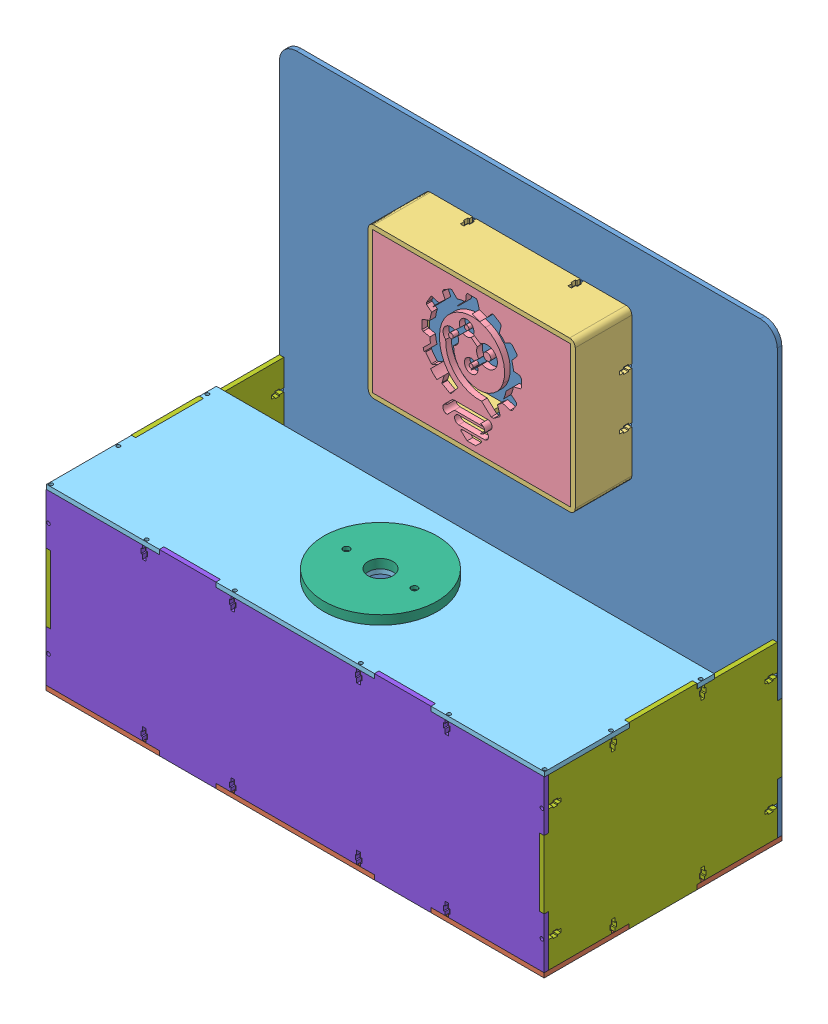
SolidWorks assembly Assemblage1, configuration Défaut. Lengths in mm.
Overall size (440.38 394 210).
10 component instances, 9 part files, 23 mates.
Components (placement in the parent):
- Pièce1-1: Pièce1 [Défaut] at origin size (440 394 4)
- Pièce2-1: Pièce2 [Défaut] at (0 -195 105) x (-1 0 0) z (0 -1 0) size (440 210 4)
- Pièce4-1: Pièce4 [Défaut] at (0 79.5409 54) x (1 0 0) z (0 0 -1) size (243.14 184.79 50)
- Part10 - Copie-1: Part10 - Copie [Default] at (-51.8221 -2.5899 50.5) size (175 125 11.52)
- Pièce7-1: Pièce7 [Défaut] at (0.3751 -41 135) x (1 0 0) z (0 -1 0) size (440 150 4)
- Pièce8-1: Pièce8 [Défaut] at (0.3751 -33 135) x (1 0 0) z (0 -1 0) size (100 100 8)
- Pièce9-1: Pièce9 [Défaut] at (-220 -120 105) x (0 0 -1) z (1 0 0) size (210 158 4)
- Pièce9-2: Pièce9 [Défaut] at (216 -120 105) x (0 0 -1) z (1 0 0) size (210 158 4)
- Pièce6-2: Pièce6 [Défaut] at (0 -120 206) size (440 158 4)
- ArduinoUno complet-1: ArduinoUno complet [Défaut] at (-169.33 -195 106.04) x (0 0 -1) z (1 0 0) size (76.34 15.58 53.34)
Mates (geometry in assembly coordinates):
- Coïncidente1: coincident anti-aligned: plane of Pièce1-1 through (220 -195 4) normal (0 -1 0); plane of Pièce2-1 through (0 -195 105) normal (0 1 0)
- Coïncidente2: coincident aligned: plane of Pièce1-1 through (0 0 0) normal (0 0 -1); plane of Pièce2-1 through (-220 -199 0) normal (0 0 -1)
- Largeur1: width aligned: plane of Pièce2-1 through (220 -199 210) normal (1 0 0); plane of Pièce2-1 through (-220 -199 210) normal (-1 0 0); plane of Pièce1-1 through (220 -195 4) normal (1 0 0); plane of Pièce1-1 through (-220 -195 4) normal (-1 0 0)
- Coïncidente5: coincident anti-aligned: plane of Pièce1-1 through (0 0 4) normal (0 0 1); plane of Pièce4-1 through (0 79.5409 4) normal (0 0 -1)
- Parallèle1: parallel aligned: plane of Pièce2-1 through (0 -195 105) normal (0 1 0); plane of Pièce4-1 through (91.5 146.0409 4) normal (0 1 0)
- Largeur2: width aligned: plane of Pièce1-1 through (-220 -195 4) normal (-1 0 0); plane of Pièce1-1 through (220 -195 4) normal (1 0 0); plane of Pièce4-1 through (-91.5 146.0409 4) normal (-1 0 0); plane of Pièce4-1 through (91.5 146.0409 4) normal (1 0 0)
- Coïncidente7: coincident anti-aligned: plane of Pièce4-1 through (-85.9962 142.0409 4) normal (0 -1 0); plane of Part10 - Copie-1 through (-87.5 142.0409 49) normal (0 1 0)
- Coïncidente8: coincident aligned: plane of Pièce4-1 through (0 79.5409 54) normal (0 0 1); plane of Part10 - Copie-1 through (-51.8221 -2.5899 54) normal (0 0 1)
- Coïncidente9: coincident: plane of Pièce4-1 through (-87.5 142.0409 4) normal (1 0 0); line of Part10 - Copie-1 through (-87.5 17.0409 54) axis (0 1 0)
- Coïncidente23: coincident anti-aligned: plane of Pièce7-1 through (0.3751 -41 135) normal (0 1 0); plane of Pièce8-1 through (0.3751 -41 135) normal (0 -1 0)
- Coaxiale1: concentric aligned: cylinder of Pièce7-1 through (0.3751 -51 135) axis (0 1 0) radius 11; cylinder of Pièce8-1 through (0.3751 -41 135) axis (0 1 0) radius 11
- Coïncidente24: coincident anti-aligned: plane of Pièce2-1 through (0 -195 105) normal (0 1 0); plane of Pièce9-1 through (-216 -195 4) normal (0 -1 0)
- Coïncidente25: coincident aligned: plane of Pièce2-1 through (-220 -199 210) normal (-1 0 0); plane of Pièce9-1 through (-220 -120 105) normal (-1 0 0)
- Coïncidente26: coincident anti-aligned: plane of Pièce1-1 through (0 0 4) normal (0 0 1); plane of Pièce9-1 through (-216 -195 4) normal (0 0 -1)
- Coïncidente29: coincident anti-aligned: plane of Pièce2-1 through (0 -195 105) normal (0 1 0); plane of Pièce9-2 through (220 -195 4) normal (0 -1 0)
- Coïncidente30: coincident aligned: plane of Pièce2-1 through (220 -199 210) normal (1 0 0); plane of Pièce9-2 through (220 -120 105) normal (1 0 0)
- Coïncidente31: coincident anti-aligned: plane of Pièce1-1 through (0 0 4) normal (0 0 1); plane of Pièce9-2 through (220 -195 4) normal (0 0 -1)
- Coïncidente32: coincident anti-aligned: plane of Pièce2-1 through (0 -195 105) normal (0 1 0); plane of Pièce6-2 through (220 -195 210) normal (0 -1 0)
- Coïncidente33: coincident aligned: plane of Pièce2-1 through (-220 -199 210) normal (0 0 1); plane of Pièce6-2 through (0 -120 210) normal (0 0 1)
- Coïncidente34: coincident aligned: plane of Pièce9-2 through (220 -120 105) normal (1 0 0); plane of Pièce6-2 through (220 -195 210) normal (1 0 0)
- Coïncidente35: coincident anti-aligned: plane of Pièce2-1 through (0 -195 105) normal (0 1 0); plane of ArduinoUno complet-1 through (-169.33 -195 106.04) normal (0 -1 0)
- Distance1: distance = 20 mm anti-aligned: plane of ArduinoUno complet-1 through (-196 -193.35 106.04) normal (-1 0 0); plane of Pièce9-1 through (-216 -120 105) normal (1 0 0)
- Distance2: distance = 60 mm anti-aligned: plane of Pièce1-1 through (0 0 4) normal (0 0 1); plane of ArduinoUno complet-1 through (-158.18 -193.35 64) normal (0 0 -1)
